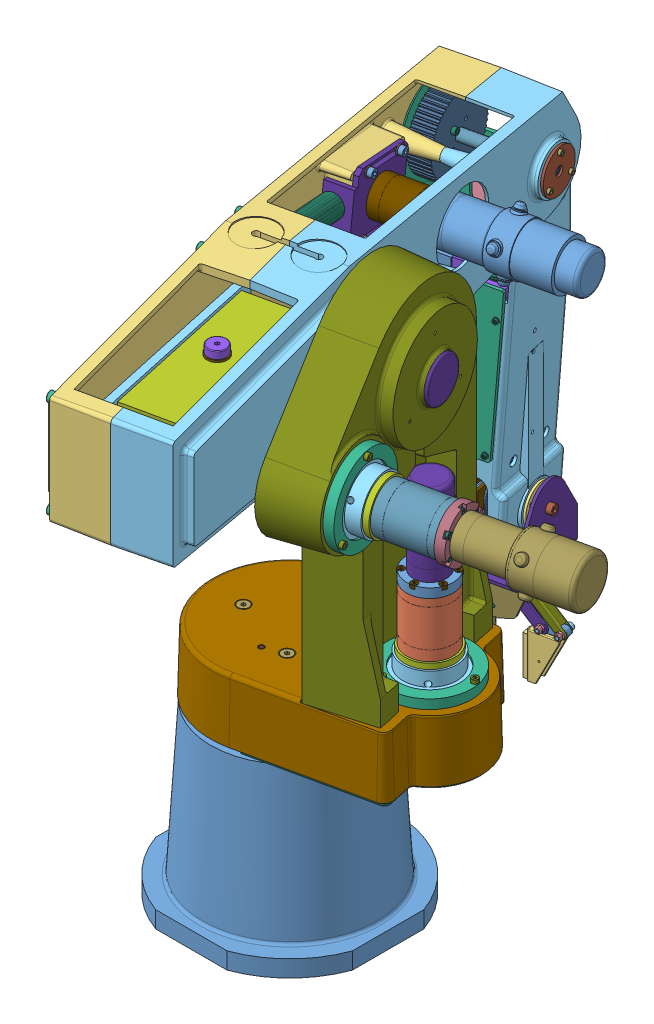
SolidWorks assembly Robot, configuration Défaut. Lengths in mm.
Overall size (506.37 616.21 601.95).
349 component instances, 132 part files, 24 mates.
Components (placement in the parent):
- Ens_Socle-1: Ens_Socle [Défaut] at origin size (212.48 231.5 219.24)
  - Socle-1: Socle [Default] at origin size (212.48 180 219.24)
  - Fourreau_200-604-1: Fourreau_200-604 [Défaut] at (0 176.5 0) x (-0.083866 0 0.996477) z (-0.996477 0 -0.083866) size (96 55 96)
  - CHC-M6_20-1: CHC-M6_20 [ISO 4762 M6 x 20 --- 20C] at (3.6062 156 -42.8485) x (0 1 0) z (-0.546944 0 0.837169) size (26 10 10)
  - poulie lacet-1: poulie lacet [Défaut] at (0 206.5 0) x (0.433454 0 0.901176) z (0 1 0) size (124 124 27)
  - Rondelle M6-1: Rondelle M6 [Washer ISO 7089 - 6] at (-35.9297 209 -24.5216) x (0 -1 0) z (0 0 1) size (1.6 12 12)
  - CHC-M6_25-1: CHC-M6_25 [ISO 4762 M6 x 25 --- 25C] at (-35.9297 216.6 -24.5216) x (0 -1 0) z (0.040163 0 0.999193) size (31 10 10)
  - Couvercle_300-732-1: Couvercle_300-732 [Défaut] at (0 175.5 0) x (-0.570868 0 0.821042) z (-0.821042 0 -0.570868) size (65 10.5 65)
  - CHC-M4_16-1: CHC-M4_16 [ISO 4762 M4 x 16 --- 16C] at (25.3374 166.5 -11.917) x (0 1 0) z (-0.937005 0 0.349316) size (20 7 7)
  - CHC-M4_16-2: CHC-M4_16 [ISO 4762 M4 x 16 --- 16C] at (-22.9892 166.5 -15.9843) x (0 1 0) z (0.771019 0 0.636812) size (20 7 7)
  - CHC-M4_16-3: CHC-M4_16 [ISO 4762 M4 x 16 --- 16C] at (-2.3482 166.5 27.9014) x (0 1 0) z (0.165986 0 -0.986128) size (20 7 7)
  - CHC-M6_25-2: CHC-M6_25 [ISO 4762 M6 x 25 --- 25C] at (-3.2715 216.6 43.3768) x (0 -1 0) z (0.845245 0 -0.534379) size (31 10 10)
  - CHC-M6_25-3: CHC-M6_25 [ISO 4762 M6 x 25 --- 25C] at (39.2011 216.6 -18.8552) x (0 -1 0) z (-0.885408 0 -0.464814) size (31 10 10)
  - Rondelle M6-2: Rondelle M6 [Washer ISO 7089 - 6] at (-3.2715 209 43.3768) x (0 -1 0) z (0.866025 0 -0.5) size (1.6 12 12)
  - Rondelle M6-3: Rondelle M6 [Washer ISO 7089 - 6] at (39.2011 209 -18.8552) x (0 -1 0) z (-0.866025 0 -0.5) size (1.6 12 12)
  - CHC-M6_20-2: CHC-M6_20 [ISO 4762 M6 x 20 --- 20C] at (-38.911 156 18.3012) x (0 1 0) z (0.998482 0 0.055083) size (26 10 10)
  - CHC-M6_20-3: CHC-M6_20 [ISO 4762 M6 x 20 --- 20C] at (35.3048 156 24.5473) x (0 1 0) z (-0.451538 0 -0.892252) size (26 10 10)
- SE_Chaise-1: SE_Chaise [Défaut] at (0 253.5 0) x (-0.212271 0 -0.977211) z (0 -1 0) size (256.43 420.65 448.71)
  - SE-Assise-1: SE-Assise [Défaut] at origin size (171.51 268.51 86)
    - Assise_100-032-1: Assise_100-032 [Default] at origin size (171.51 268.51 67)
    - Axe_200-464-1: Axe_200-464 [Défaut] at (0 0 11.5) x (0 0 1) z (1 0 0) size (76 96 96)
    - Goupille élastique , 6x20-1: Goupille élastique , 6x20 [Défaut] at (-40 0 10) x (1 0 0) z (0 -1 0) size (5.98 20 6)
    - Goupille élastique , 6x20-2: Goupille élastique , 6x20 [Défaut] at (40 0 10) x (1 0 0) z (0 -1 0) size (5.98 20 6)
    - visFHC M6-16-1: visFHC M6-16 [B18.3.5M - 6 x 1.0 x 16 Socket FCHS  -- 16S] at (0 -42 0) x (0 0 1) z (-1 0 0) size (16 11.7 11.7)
    - visFHC M6-16-2: visFHC M6-16 [B18.3.5M - 6 x 1.0 x 16 Socket FCHS  -- 16S] at (-36.3731 21 0) x (0 0 1) z (0.5 0.866025 0) size (16 11.7 11.7)
    - visFHC M6-16-3: visFHC M6-16 [B18.3.5M - 6 x 1.0 x 16 Socket FCHS  -- 16S] at (36.3731 21 0) x (0 0 1) z (0.5 -0.866025 0) size (16 11.7 11.7)
    - SKF_7204-1: SKF_7204 [SKF - 7204 BE - 10,DE,NC,10_68] at (0 0 31) x (0 0 1) z (-1 0 0) size (14 47 47)
    - SKF_7204-2: SKF_7204 [SKF - 7204 BE - 10,DE,NC,10_68] at (0 0 67.5) x (0 0 -1) z (1 0 0) size (14 47 47)
    - Entrtoise_200-006-1: Entrtoise_200-006 [Default] at (0 0 38) x (1 0 0) z (0 -1 0) size (47 22.5 47)
    - Capot_201-294-1: Capot_201-294 [Défaut] at (0 0.5 67) size (170 180.5 2)
  - Dossier-1: Dossier [Défaut] at (-0.0064 64.9972 -279) x (1 0 0) z (0 1 0) size (234.27 388.58 71.5)
  - Moto-réducteur lacet-1: Moto-réducteur lacet [Défaut] at (2.5917 125.4972 -183.1) x (0 0 -1) z (0.5 0.866025 0) size (236.28 90 90)
    - Corps moto-réducteur-1: Corps moto-réducteur [Default] at origin size (199.6 50 51)
      - Moteur Parvex RS120G-1: Moteur Parvex RS120G [Défaut] at origin size (126 39.96 39.96)
      - Vis CHC M4x10-1: Vis CHC M4x10 [Défaut] at (-91.1 0 22) x (0 0 1) z (-1 0 0) size (7 7 14)
      - Entretoise-m-r-1: Entretoise-m-r [Défaut] at (-92.6 0 0) size (59.8 50 50)
      - Réducteur Harmonic Drive HDUC 14 1U-CC-1: Réducteur Harmonic Drive HDUC 14 1U-CC [Défaut] at (-92.6 0 0) size (123.2 50 50)
      - Vis CHC M4x10-2: Vis CHC M4x10 [Défaut] at (-91.1 -19.0526 11) x (0 -0.866025 0.5) z (-1 0 0) size (7 7 14)
      - Vis CHC M4x10-3: Vis CHC M4x10 [Défaut] at (-91.1 -19.0526 -11) x (0 -0.866025 -0.5) z (-1 0 0) size (7 7 14)
      - Vis CHC M4x10-4: Vis CHC M4x10 [Défaut] at (-91.1 0 -22) x (0 0 -1) z (-1 0 0) size (7 7 14)
      - Vis CHC M4x10-5: Vis CHC M4x10 [Défaut] at (-91.1 19.0526 -11) x (0 0.866025 -0.5) z (-1 0 0) size (7 7 14)
      - Vis CHC M4x10-6: Vis CHC M4x10 [Défaut] at (-91.1 19.0526 11) x (0 0.866025 0.5) z (-1 0 0) size (7 7 14)
      - Vis CHC M4-6-1: Vis CHC M4-6 [Défaut] at (-90.1 9.8995 9.8995) x (0 0 -1) z (1 0 0) size (6 6 10)
      - Vis CHC M4-6-2: Vis CHC M4-6 [Défaut] at (-90.1 -9.8995 9.8995) x (0 1 0) z (1 0 0) size (6 6 10)
      - Vis CHC M4-6-3: Vis CHC M4-6 [Défaut] at (-90.1 -9.8995 -9.8995) x (0 0 1) z (1 0 0) size (6 6 10)
      - Vis CHC M4-6-4: Vis CHC M4-6 [Défaut] at (-90.1 9.8995 -9.8995) x (0 -1 0) z (1 0 0) size (6 6 10)
      - Arbre de sortie-1: Arbre de sortie [Défaut] at (-159.6 0 0) size (40 8 8)
    - Palier-1: Palier [Défaut] at (-162.6 0 0) size (88.18 90 90)
      - Porte poulie motrice-1: Porte poulie motrice [Défaut] at origin size (73.68 74 74)
      - Bride-1: Bride [Défaut] at (-22.5 3 0) x (0 0 -1) z (-1 0 0) size (90 90 10)
      - Flasque-1: Flasque [Défaut] at (6 0 0) x (0 -0.664186 0.747567) z (-1 0 0) size (54 54 6)
      - VisCHC M4-40-1: VisCHC M4-40 [Défaut] at (-36 -16.2635 16.2635) x (0 0.997296 -0.073485) z (1 0 0) size (7 7 44)
      - VisCHC M4-40-2: VisCHC M4-40 [Défaut] at (-36 16.2635 16.2635) x (0 -0.073485 -0.997296) z (1 0 0) size (7 7 44)
      - VisCHC M4-40-3: VisCHC M4-40 [Défaut] at (-36 16.2635 -16.2635) x (0 -0.997296 0.073485) z (1 0 0) size (7 7 44)
      - VisCHC M4-40-4: VisCHC M4-40 [Défaut] at (-36 -16.2635 -16.2635) x (0 0.073485 0.997296) z (1 0 0) size (7 7 44)
      - anneau élastique int d32-1: anneau élastique int d32 [Défaut] at (-48.6 0 0) x (0 0 1) z (-1 0 0) size (33.7 32.99 1.2)
      - Vis CHC M4x10-1: Vis CHC M4x10 [Défaut] at (4.5 20 0) x (0 0 -1) z (1 0 0) size (7 7 14)
      - Vis CHC M4x10-2: Vis CHC M4x10 [Défaut] at (4.5 10 17.3205) x (0 0.866025 -0.5) z (1 0 0) size (7 7 14)
      - Vis CHC M4x10-3: Vis CHC M4x10 [Défaut] at (4.5 -10 17.3205) x (0 0.866025 0.5) z (1 0 0) size (7 7 14)
      - Vis CHC M4x10-4: Vis CHC M4x10 [Défaut] at (4.5 -20 0) x (0 0 1) z (1 0 0) size (7 7 14)
      - Vis CHC M4x10-5: Vis CHC M4x10 [Défaut] at (4.5 -10 -17.3205) x (0 -0.866025 0.5) z (1 0 0) size (7 7 14)
      - Vis CHC M4x10-6: Vis CHC M4x10 [Défaut] at (4.5 10 -17.3205) x (0 -0.866025 -0.5) z (1 0 0) size (7 7 14)
    - SKF 6002-1: SKF 6002 [SKF - 6002 - 12,DE,NC,12_68] at (-206.7 0 0) size (9 32 32)
    - SKF 6002-2: SKF 6002 [SKF - 6002 - 12,DE,NC,12_68] at (-185.6 0 0) size (9 32 32)
  - vis CHC M6-25-1: vis CHC M6-25 [ISO 4762 M6 x 25 --- 25S] at (-57.0064 122.9972 16) x (0 0 -1) z (-0.036606 -0.99933 0) size (31 10 10)
  - vis CHC M6-25-2: vis CHC M6-25 [ISO 4762 M6 x 25 --- 25S] at (-57.0064 77.9972 16) x (0 0 -1) z (-0.036606 -0.99933 0) size (31 10 10)
  - vis CHC M6-25-3: vis CHC M6-25 [ISO 4762 M6 x 25 --- 25S] at (56.9936 122.9972 16) x (0 0 -1) z (-0.036606 -0.99933 0) size (31 10 10)
  - vis CHC M6-25-4: vis CHC M6-25 [ISO 4762 M6 x 25 --- 25S] at (56.9936 77.9972 16) x (0 0 -1) z (-0.036606 -0.99933 0) size (31 10 10)
  - Goupille élastique , 6x20-1: Goupille élastique , 6x20 [Défaut] at (66.9936 122.9972 2) x (1 0 0) z (0 -1 0) size (5.98 20 6)
  - Goupille élastique , 6x20-2: Goupille élastique , 6x20 [Défaut] at (-42.0064 77.9972 2) x (1 0 0) z (0 -1 0) size (5.98 20 6)
  - Moteur Epaule-1: Moteur Epaule [Défaut] at (-95.2692 334.8972 -221) x (0 1 0) z (0.162984 0 0.986629) size (264.08 126.67 126.67)
    - Moteur RS210-1: Moteur RS210 [Défaut] at origin size (135.4 52 52)
    - entretoise-m-r bras-1: entretoise-m-r bras [Défaut] at (-120.4 0 0) x (1 0 0) z (0 0.162984 0.986629) size (59.8 54 54)
    - Réducteur Harmonic Drive bras-1: Réducteur Harmonic Drive bras [Défaut] at (-120.4 0 0) x (1 0 0) z (0 0.634463 0.772953) size (123.2 51.79 50)
    - Vis CHC M4x10-1: Vis CHC M4x10 [Défaut] at (-117.9 11.3806 8.1537) x (0 0.924309 0.381646) z (1 0 0) size (7 7 14)
    - Vis CHC M4x10-2: Vis CHC M4x10 [Défaut] at (-117.9 -8.1537 11.3806) x (0 -0.381646 0.924309) z (1 0 0) size (7 7 14)
    - Vis CHC M4x10-3: Vis CHC M4x10 [Défaut] at (-117.9 -11.3806 -8.1537) x (0 -0.924309 -0.381646) z (1 0 0) size (7 7 14)
    - Vis CHC M4x10-4: Vis CHC M4x10 [Défaut] at (-117.9 8.1537 -11.3806) x (0 0.381646 -0.924309) z (1 0 0) size (7 7 14)
    - Vis CHC M3-10-1: Vis CHC M3-10 [Défaut] at (-118.9 3.5857 21.7058) x (0 -0.692088 -0.721813) z (-1 0 0) size (5.5 5.5 13)
    - Vis CHC M3-10-2: Vis CHC M3-10 [Défaut] at (-118.9 -17.005 13.9582) x (0 0.279064 -0.960272) z (-1 0 0) size (5.5 5.5 13)
    - Vis CHC M3-10-3: Vis CHC M3-10 [Défaut] at (-118.9 -20.5906 -7.7476) x (0 0.971152 -0.238459) z (-1 0 0) size (5.5 5.5 13)
    - Vis CHC M3-10-4: Vis CHC M3-10 [Défaut] at (-118.9 -3.5857 -21.7058) x (0 0.692088 0.721813) z (-1 0 0) size (5.5 5.5 13)
    - Vis CHC M3-10-5: Vis CHC M3-10 [Défaut] at (-118.9 17.005 -13.9582) x (0 -0.279064 0.960272) z (-1 0 0) size (5.5 5.5 13)
    - Vis CHC M3-10-6: Vis CHC M3-10 [Défaut] at (-118.9 20.5906 7.7476) x (0 -0.971152 0.238459) z (-1 0 0) size (5.5 5.5 13)
    - Palier-1: Palier [Défaut] at (-190.4 0 0) x (1 0 0) z (0 0.634463 0.772953) size (88.18 90 90)
      - Porte poulie motrice-1: Porte poulie motrice [Défaut] at origin size (73.68 74 74)
      - Bride-1: Bride [Défaut] at (-22.5 3 0) x (0 0 -1) z (-1 0 0) size (90 90 10)
      - Flasque-1: Flasque [Défaut] at (6 0 0) x (0 -0.664186 0.747567) z (-1 0 0) size (54 54 6)
      - VisCHC M4-40-1: VisCHC M4-40 [Défaut] at (-36 -16.2635 16.2635) x (0 0.997296 -0.073485) z (1 0 0) size (7 7 44)
      - VisCHC M4-40-2: VisCHC M4-40 [Défaut] at (-36 16.2635 16.2635) x (0 -0.073485 -0.997296) z (1 0 0) size (7 7 44)
      - VisCHC M4-40-3: VisCHC M4-40 [Défaut] at (-36 16.2635 -16.2635) x (0 -0.997296 0.073485) z (1 0 0) size (7 7 44)
      - VisCHC M4-40-4: VisCHC M4-40 [Défaut] at (-36 -16.2635 -16.2635) x (0 0.073485 0.997296) z (1 0 0) size (7 7 44)
      - anneau élastique int d32-1: anneau élastique int d32 [Défaut] at (-48.6 0 0) x (0 0 1) z (-1 0 0) size (33.7 32.99 1.2)
      - Vis CHC M4x10-1: Vis CHC M4x10 [Défaut] at (4.5 20 0) x (0 0 -1) z (1 0 0) size (7 7 14)
      - Vis CHC M4x10-2: Vis CHC M4x10 [Défaut] at (4.5 10 17.3205) x (0 0.866025 -0.5) z (1 0 0) size (7 7 14)
      - Vis CHC M4x10-3: Vis CHC M4x10 [Défaut] at (4.5 -10 17.3205) x (0 0.866025 0.5) z (1 0 0) size (7 7 14)
      - Vis CHC M4x10-4: Vis CHC M4x10 [Défaut] at (4.5 -20 0) x (0 0 1) z (1 0 0) size (7 7 14)
      - Vis CHC M4x10-5: Vis CHC M4x10 [Défaut] at (4.5 -10 -17.3205) x (0 -0.866025 0.5) z (1 0 0) size (7 7 14)
      - Vis CHC M4x10-6: Vis CHC M4x10 [Défaut] at (4.5 10 -17.3205) x (0 -0.866025 -0.5) z (1 0 0) size (7 7 14)
    - SKF 6002-1: SKF 6002 [SKF - 6002 - 12,DE,NC,12_68] at (-213.4 0 0) size (9 32 32)
    - SKF 6002-2: SKF 6002 [SKF - 6002 - 12,DE,NC,12_68] at (-234.5 0 0) size (9 32 32)
  - Vis_CHC_M4-16-1: Vis_CHC_M4-16 [ISO 4762 M4 x 12 --- 12C] at (-133.3743 135.9972 -202) x (0 -1 0) z (0 0 1) size (20 7 7)
  - Vis_CHC_M4-16-2: Vis_CHC_M4-16 [ISO 4762 M4 x 12 --- 12C] at (-0.0064 167.9972 -12) x (0 0 1) z (0 1 0) size (20 7 7)
  - Vis_CHC_M4-16-3: Vis_CHC_M4-16 [ISO 4762 M4 x 12 --- 12C] at (-35.5134 106.4972 -12) x (0 0 1) z (-0.866025 -0.5 0) size (20 7 7)
  - Vis_CHC_M4-16-4: Vis_CHC_M4-16 [ISO 4762 M4 x 12 --- 12C] at (35.5007 106.4972 -12) x (0 0 1) z (0.866025 -0.5 0) size (20 7 7)
  - Vis_CHC_M4-16-5: Vis_CHC_M4-16 [ISO 4762 M4 x 12 --- 12C] at (-97.8672 135.9972 -263.5) x (0 -1 0) z (-0.866025 0 -0.5) size (20 7 7)
  - Vis_CHC_M4-16-6: Vis_CHC_M4-16 [ISO 4762 M4 x 12 --- 12C] at (-62.3602 135.9972 -202) x (0 -1 0) z (0.866025 0 -0.5) size (20 7 7)
  - Bouchon-1: Bouchon [Défaut] at (-0.0064 133.9972 -279) size (46 5.5 46)
  - Couvercle_301-396-1: Couvercle_301-396 [Défaut] at (-0.0064 71.9972 -279) x (0.866025 0 0.5) z (-0.5 0 0.866025) size (66 8 66)
  - Vis_CHC_M4-16-7: Vis_CHC_M4-16 [ISO 4762 M4 x 12 --- 12C] at (-0.0064 71.9972 -307.5) x (0 1 0) z (-0.976883 0 -0.213777) size (20 7 7)
  - Vis_CHC_M4-16-8: Vis_CHC_M4-16 [ISO 4762 M4 x 12 --- 12C] at (-24.6881 71.9972 -264.75) x (0 1 0) z (0.303305 0 0.952894) size (20 7 7)
  - Vis_CHC_M4-16-9: Vis_CHC_M4-16 [ISO 4762 M4 x 12 --- 12C] at (24.6754 71.9972 -264.75) x (0 1 0) z (0.673578 0 -0.739117) size (20 7 7)
  - Ecrou à encoches, M 17-1: Ecrou à encoches, M 17 [Défaut] at (0 0 75.5) x (-0.99693 -0.078302 0) z (-0.078302 0.99693 0) size (27.71 5 27.71)
  - Rondelle frein de 17-1: Rondelle frein de 17 [Défaut] at (0 0 74.5) x (-0.99693 -0.078302 0) z (-0.078302 0.99693 0) size (33.42 5.39 32.18)
- Bras-1: Bras [Défaut] at (-0.5391 505.7717 6.953) x (0.212271 0 0.977211) z (-0.977211 0 0.212271) size (576.57 148.84 242.4)
  - BrasDroit-2: BrasDroit [Défaut] at origin size (576.57 148.84 66)
  - GoupillePosition-1: GoupillePosition [Défaut] at (-30.6737 92.2283 0) x (0 0 1) z (-1 0 0) size (10 8 8)
  - GoupillePosition-3: GoupillePosition [Défaut] at (234.3263 -27.2717 0) x (0 0 1) z (-1 0 0) size (10 8 8)
  - GoupillePosition-4: GoupillePosition [Défaut] at (-227.6737 51.7283 0) x (0 0 1) z (-1 0 0) size (10 8 8)
  - BrasGauche-2: BrasGauche [Défaut] at (-6.6737 26.7283 0) size (576.57 148.84 101.36)
  - Vis C HC, M 6x70-1: Vis C HC, M 6x70 [Défaut] at (-227.6737 51.7283 55) x (-0.629032 0.777379 0) z (0.777379 0.629032 0) size (10 76 10)
  - Vis C HC, M 6x70-7: Vis C HC, M 6x70 [Défaut] at (-30.6737 92.2283 55) x (0.427468 -0.90403 0) z (-0.90403 -0.427468 0) size (10 76 10)
  - Vis C HC, M 6x70-9: Vis C HC, M 6x70 [Défaut] at (234.3263 -27.2717 55) x (0.427468 -0.90403 0) z (-0.90403 -0.427468 0) size (10 76 10)
  - Vis C HC, M 6x70-11: Vis C HC, M 6x70 [Défaut] at (-165.6737 -17.2717 55) x (0.427468 -0.90403 0) z (-0.90403 -0.427468 0) size (10 76 10)
  - Vis C HC, M 6x70-15: Vis C HC, M 6x70 [Défaut] at (234.3263 77.7283 55) x (0.427468 -0.90403 0) z (-0.90403 -0.427468 0) size (10 76 10)
  - Vis C HC, M 6x70-21: Vis C HC, M 6x70 [Défaut] at (23.3263 91.126 55) x (0.427468 -0.90403 0) z (-0.90403 -0.427468 0) size (10 76 10)
  - Vis C HC, M 6x70-23: Vis C HC, M 6x70 [Défaut] at (-6.6737 -38.7717 55) x (0.427468 -0.90403 0) z (-0.90403 -0.427468 0) size (10 76 10)
  - contre_poids-1: contre_poids [Défaut] at (123.9539 42.7283 -46) size (175 60 60)
  - Vis C HC, M 8x70-1: Vis C HC, M 8x70 [Défaut] at (117.4539 78.7283 -16) x (0.870431 0 -0.492291) z (0.492291 0 0.870431) size (20 78.34 20)
  - Rondelle L, 8-1: Rondelle L, 8 [Défaut] at (117.4539 75.7283 -16) size (22 1.5 22)
  - Rondelle L, 8-3: Rondelle L, 8 [Défaut] at (117.4539 77.2283 -16) size (22 1.5 22)
  - SKF_6001-1: SKF_6001 [SKF - 6001 - 10,DE,NC,10_68] at (-286.6737 26.7283 -58) x (0 0 -1) z (1 0 0) size (8 28 28)
  - Couvercle_M300-013-1: Couvercle_M300-013 [Défaut] at (-286.6737 26.7283 -64) x (0 0 1) z (-1 0 0) size (4.5 45 45)
  - CHC_M3-10-1: CHC_M3-10 [ISO 4762 M3 x 10 --- 10C] at (-302.2622 17.7283 -69.5) x (0 0 1) z (-1 0 0) size (13 5.5 5.5)
  - CHC_M3-10-3: CHC_M3-10 [ISO 4762 M3 x 10 --- 10C] at (-286.6737 44.7283 -69.5) x (0 0 1) z (-1 0 0) size (13 5.5 5.5)
  - CHC_M3-10-9: CHC_M3-10 [ISO 4762 M3 x 10 --- 10C] at (-271.0852 17.7283 -69.5) x (0 0 1) z (-1 0 0) size (13 5.5 5.5)
  - Verin-pince-1: Verin-pince [Défaut] at (-48.6737 7.2342 -0.5445) x (-1 0 0) z (0 -0.130938 0.991391) size (269.69 47.71 50)
    - Support-verin-1: Support-verin [Défaut] at origin size (170 44 50)
    - 5079 DSN-25-80-1: 5079 DSN-25-80 [Défaut] at (-118.1875 36.1693 13.898) x (0 -0.972057 -0.234746) z (1 0 0) size (36.95 32 205.57)
      - Corps-1: Corps [Défaut] at (13.1476 11.1224 0) size (27 27 173.5)
      - Piston-1: Piston [Défaut] at (13.1476 11.1224 4.0685) size (25 25 177.5)
      - Ecrou-1: Ecrou [Défaut] at (13.1476 11.1224 2.0036) size (36.95 32 11)
  - CHC_M3-10-10: CHC_M3-10 [ISO 4762 M3 x 10 --- 10C] at (106.3263 -1.975 9.6121) x (0 0.991391 0.130938) z (0 -0.130938 0.991391) size (13 5.5 5.5)
  - CHC_M3-10-11: CHC_M3-10 [ISO 4762 M3 x 10 --- 10C] at (106.3263 0.8402 -11.7028) x (0 0.991391 0.130938) z (-0.130938 -0.129811 0.982855) size (13 5.5 5.5)
  - SupportMoteur_M300-005-1: SupportMoteur_M300-005 [Défaut] at (-166.3149 43.5192 23.5) x (-0.988512 -0.151141 0) z (0 0 -1) size (75 70 28)
  - Rondelle Z, 3-1: Rondelle Z, 3 [Défaut] at (106.3263 0.9992 10.0049) x (1 0 0) z (0 -0.130938 0.991391) size (6 0.8 6)
  - Rondelle Z, 3-3: Rondelle Z, 3 [Défaut] at (106.3263 3.8144 -11.31) x (1 0 0) z (0 -0.130938 0.991391) size (6 0.8 6)
  - VisCHC_M5-16-1: VisCHC_M5-16 [ISO 4762 M5 x 16 --- 16C] at (-149.3329 75.8068 12.5) x (0 0 1) z (-0.747365 -0.664413 0) size (21 8.5 8.5)
  - VisCHC_M5-16-3: VisCHC_M5-16 [ISO 4762 M5 x 16 --- 16C] at (-141.3413 15.8945 12.5) x (0 0 1) z (-1 0 0) size (21 8.5 8.5)
  - VisCHC_M5-16-5: VisCHC_M5-16 [ISO 4762 M5 x 16 --- 16C] at (-185.0651 10.9723 12.5) x (0 0 1) z (-1 0 0) size (21 8.5 8.5)
  - VisCHC_M5-16-7: VisCHC_M5-16 [ISO 4762 M5 x 16 --- 16C] at (-193.005 70.4446 12.5) x (0 0 1) z (-1 0 0) size (21 8.5 8.5)
  - Rondelle Z, 5-1: Rondelle Z, 5 [Défaut] at (-185.0651 10.9723 18.5) x (1 0 0) z (0 1 0) size (10 1 10)
  - Rondelle Z, 5-3: Rondelle Z, 5 [Défaut] at (-193.005 70.4446 18.5) x (1 0 0) z (0 1 0) size (10 1 10)
  - Rondelle Z, 5-5: Rondelle Z, 5 [Défaut] at (-149.3329 75.8068 18.5) x (1 0 0) z (0 1 0) size (10 1 10)
  - Rondelle Z, 5-7: Rondelle Z, 5 [Défaut] at (-141.3413 15.8945 18.5) x (1 0 0) z (0 1 0) size (10 1 10)
  - AXE_Bras-1: AXE_Bras [Défaut] at (-6.6737 26.7283 -80) x (0 0 -1) z (-1 0 0) size (72.5 126.04 126.04)
    - AXE_M300-010-1: AXE_M300-010 [Défaut] at origin size (72.5 98 98)
    - Poulie_M300-014-1: Poulie_M300-014 [Défaut] at (-4 0 0) size (30 126.04 126.04)
    - Vic_CHCM6-16-1: Vic_CHCM6-16 [ISO 4762 M6 x 16 --- 16C] at (9.2 22 -38.1051) x (-1 0 0) z (0 0.831566 -0.555426) size (22 10 10)
    - Goupille6-32-1: Goupille6-32 [Parallel Pin ISO 8734 - 6 x 32 - A - St] at (-14 44 0) size (32 6 6)
    - Goupille6-32-2: Goupille6-32 [Parallel Pin ISO 8734 - 6 x 32 - A - St] at (-14 -31.1127 31.1127) x (1 0 0) z (0 -0.90193 0.431882) size (32 6 6)
    - EntretoiseM200-006-1: EntretoiseM200-006 [Défaut] at (35.5 0 0) x (1 0 0) z (0 -0.984877 -0.173252) size (21.5 47 47)
    - 7204_Rlt-Billes-1: 7204_Rlt-Billes [SKF - 7204 BE - 10,DE,NC,10_68] at (7 0 0) x (1 0 0) z (0 -0.825996 0.563676) size (14 47 47)
    - 7204_Rlt-Billes-2: 7204_Rlt-Billes [SKF - 7204 BE - 10,DE,NC,10_68] at (42.5 0 0) x (-1 0 0) z (0 -0.662732 0.748856) size (14 47 47)
    - Ecrou à encoches, M 20-1: Ecrou à encoches, M 20 [Défaut] at (50.5 0 0) x (0 0.493503 -0.869744) z (0 -0.869744 -0.493503) size (31.75 7.06 31.75)
    - Rondelle frein de 20-1: Rondelle frein de 20 [Défaut] at (49.5 0 0) x (0 0.317084 0.948397) z (0 0.948397 -0.317084) size (36.64 6.14 35.22)
    - Rondelle M, 6-1: Rondelle M, 6 [Défaut] at (2 22 -38.1051) x (0 -0.99765 -0.068521) z (0 -0.068521 0.99765) size (14 1.2 14)
    - Vic_CHCM6-16-2: Vic_CHCM6-16 [ISO 4762 M6 x 16 --- 16C] at (9.2 -44 0) x (-1 0 0) z (0 -0.896796 -0.442445) size (22 10 10)
    - Vic_CHCM6-16-3: Vic_CHCM6-16 [ISO 4762 M6 x 16 --- 16C] at (9.2 22 38.1051) x (-1 0 0) z (0 0.06523 0.99787) size (22 10 10)
    - Rondelle M, 6-2: Rondelle M, 6 [Défaut] at (2 -44 0) x (0 0.439484 0.89825) z (0 0.89825 -0.439484) size (14 1.2 14)
    - Rondelle M, 6-3: Rondelle M, 6 [Défaut] at (2 22 38.1051) x (0 0.558165 -0.82973) z (0 -0.82973 -0.558165) size (14 1.2 14)
  - Rondelle M, 6-1: Rondelle M, 6 [Défaut] at (-6.6737 -3.0038 -59) x (1 0 0) z (0 -1 0) size (14 1.2 14)
  - Rondelle M, 6-3: Rondelle M, 6 [Défaut] at (-32.4225 41.5944 -59) x (1 0 0) z (0 -1 0) size (14 1.2 14)
  - Rondelle M, 6-5: Rondelle M, 6 [Défaut] at (19.0751 41.5944 -59) x (1 0 0) z (0 -1 0) size (14 1.2 14)
  - Vic_CHCM6-16-7: Vic_CHCM6-16 [ISO 4762 M6 x 16 --- 16C] at (-32.4225 41.5944 -51.8) x (0 0 -1) z (1 0 0) size (22 10 10)
  - Vic_CHCM6-16-9: Vic_CHCM6-16 [ISO 4762 M6 x 16 --- 16C] at (-6.6737 -3.0038 -51.8) x (0 0 -1) z (1 0 0) size (22 10 10)
  - Vic_CHCM6-16-11: Vic_CHCM6-16 [ISO 4762 M6 x 16 --- 16C] at (19.0751 41.5944 -51.8) x (0 0 -1) z (-1 0 0) size (22 10 10)
  - parallel pin unhardened_iso-1: parallel pin unhardened_iso [Parallel Pin ISO 2338 - 6 m6 x 20 - St] at (-6.6737 56.7283 -73) x (0 0 1) z (0.997282 0.073675 0) size (20 6 6)
  - parallel pin unhardened_iso-3: parallel pin unhardened_iso [Parallel Pin ISO 2338 - 6 m6 x 20 - St] at (14.5395 5.5151 -73) x (0 0 1) z (0.997282 0.073675 0) size (20 6 6)
  - Couvercle_M300-013-4: Couvercle_M300-013 [Défaut] at (-286.6737 26.7283 63) x (0 0 -1) z (1 0 0) size (4.5 45 45)
  - Rondelle épaisse Z, 12-1: Rondelle épaisse Z, 12 [Défaut] at (-286.6737 26.7283 -50.5) x (0.066998 0.997753 0) z (-0.997753 0.066998 0) size (15 3.5 15)
  - SKF_6001-2: SKF_6001 [SKF - 6001 - 10,DE,NC,10_68] at (-286.6737 26.7283 57) x (0 0 -1) z (0.798379 0.602155 0) size (8 28 28)
  - Rondelle épaisse Z, 12-3: Rondelle épaisse Z, 12 [Défaut] at (-286.6737 26.7283 49.5) x (0.444076 -0.895989 0) z (-0.895989 -0.444076 0) size (15 3.5 15)
  - CHC_M3-10-14: CHC_M3-10 [ISO 4762 M3 x 10 --- 10C] at (-271.0852 17.7283 68.5) x (0 0 -1) z (1 0 0) size (13 5.5 5.5)
  - CHC_M3-10-16: CHC_M3-10 [ISO 4762 M3 x 10 --- 10C] at (-302.2622 17.7283 68.5) x (0 0 -1) z (1 0 0) size (13 5.5 5.5)
  - CHC_M3-10-18: CHC_M3-10 [ISO 4762 M3 x 10 --- 10C] at (-286.6737 44.7283 68.5) x (0 0 -1) z (1 0 0) size (13 5.5 5.5)
  - AXE 04 021 M300 011-1: AXE 04 021 M300 011 [Défaut] at (-286.6737 26.7283 -63) x (-0.545711 0.837974 0) z (0 0 1) size (12 12 125)
  - Vis à bille M6-40-1: Vis à bille M6-40 [Défaut] at (-37.2131 63.2586 37.5) x (-0.988512 -0.151141 0) z (0.079359 -0.519031 0.851063) size (106.14 36 36)
    - socket head cap screw_iso-1: socket head cap screw_iso [PreviewCfg] at origin size (104 36 36)
    - Bille-1: Bille [Défaut] at (103.5 0 0) x (-0.326721 -0.900194 0.28793) z (-0.943911 0.295385 -0.147577) size (4 4 4)
  - hex nut gradec_iso-1: hex nut gradec_iso [Hexagon Nut ISO - 4034 - M6 - N] at (-120.7445 50.4869 37.5) x (0.022844 -0.149405 -0.988512) z (0.988512 0.151141 0) size (10 11.55 6.1)
  - MotoReduc_Coude-1: MotoReduc_Coude [Défaut] at (-166.3149 43.5192 -32.5) x (0 0 -1) z (0.805857 -0.592111 0) size (233.4 63.14 63.14)
    - Réducteur Harmonic Drive HDUC 11 1U-CC-1: Réducteur Harmonic Drive HDUC 11 1U-CC [Défaut] at origin size (123.2 40 40)
    - Moteur Parvex RS220F-1: Moteur Parvex RS220F [Défaut] at (141.4 0 0) x (1 0 0) z (0 0.244629 0.969617) size (210.51 52 52)
    - BrideCoude-1: BrideCoude [Défaut] at (-5 0 0) size (10 52 52)
    - Sortie reduc-1: Sortie reduc [Défaut] at (-52 0 0) size (40 10 10)
  - socket head cap screw_iso-1: socket head cap screw_iso [ISO 4762 M4 x 8 --- 8N] at (-149.016 46.1642 27) x (0 0 -1) z (0.779732 0.626114 0) size (12 7 7)
  - Rondelle, W 4-1: Rondelle, W 4 [Défaut] at (-149.016 46.1642 23) x (0 -1 0) z (1 0 0) size (7.3 1.5 7.3)
  - Rondelle, W 4-2: Rondelle, W 4 [Défaut] at (-168.9599 60.8182 23) x (1 0 0) z (0 1 0) size (7.3 1.5 7.3)
  - Rondelle, W 4-3: Rondelle, W 4 [Défaut] at (-183.6139 40.8743 23) x (0 1 0) z (-1 0 0) size (7.3 1.5 7.3)
  - Rondelle, W 4-4: Rondelle, W 4 [Défaut] at (-163.67 26.2203 23) x (-1 0 0) z (0 -1 0) size (7.3 1.5 7.3)
  - socket head cap screw_iso-2: socket head cap screw_iso [ISO 4762 M4 x 8 --- 8N] at (-168.9599 60.8182 27) x (0 0 -1) z (-0.626114 0.779732 0) size (12 7 7)
  - socket head cap screw_iso-3: socket head cap screw_iso [ISO 4762 M4 x 8 --- 8N] at (-183.6139 40.8743 27) x (0 0 -1) z (-0.779732 -0.626114 0) size (12 7 7)
  - socket head cap screw_iso-4: socket head cap screw_iso [ISO 4762 M4 x 8 --- 8N] at (-163.67 26.2203 27) x (0 0 -1) z (0.626114 -0.779732 0) size (12 7 7)
